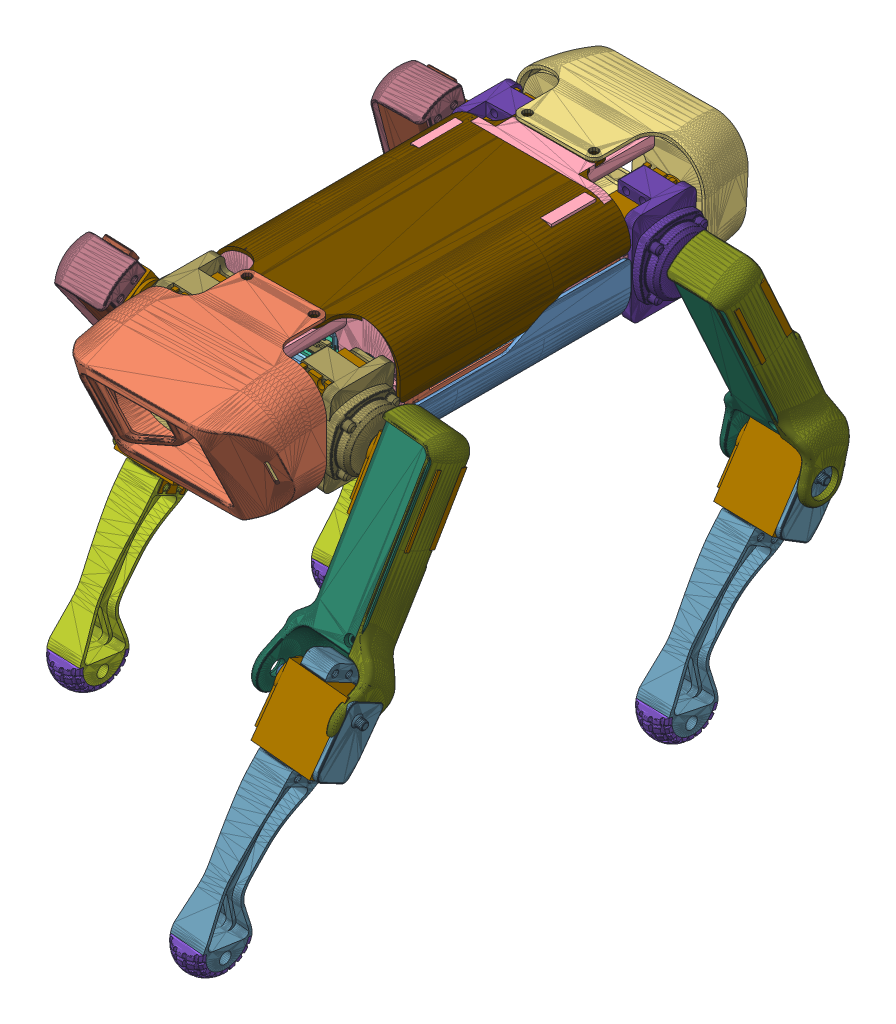
SolidWorks assembly robot_dog_jestson, configuration Default. Lengths in mm. (continued)
Components (placement in the parent): (continued)
- torsol_with_jestson-1: torsol_with_jestson [Default] at (84.8958 -47.9637 220.9974) size (110.41 70.14 242.41) (continued)
  - plate_with_jetson-1: plate_with_jetson [Default] at (-139.2728 38.0458 18.6623) x (-1 0 0) z (0 -1 0) size (107 130 44.9) (continued)
    - Jetson nano_fixed.step-1: Jetson nano_fixed.step [Default] at (-69.1681 -65.6237 -1.45) x (0 1 0) z (0 0 -1) size (100 81.03 30.51) (continued)
      - 142-13449-1000-A02_ASM.step-1: 142-13449-1000-A02_ASM.step [Default] at origin size (100 81.03 23.19) (continued)
        - 115-1821-000_1.step-2: 115-1821-000_1.step [Default] at (6.25 39.55 1.575) x (0 -1 0) z (0 0 1) size (2 2.88 1.1)
        - 115-0742-000_2.step-1: 115-0742-000_2.step [Default] at (3.05 46.85 1.575) size (2 2.88 1.1)
        - 115-0742-000_2.step-2: 115-0742-000_2.step [Default] at (3.05 51.65 1.575) x (-1 0 0) z (0 0 1) size (2 2.88 1.1)
        - 115-1821-000_1.step-3: 115-1821-000_1.step [Default] at (59.6 27.6 1.575) x (0 1 0) z (0 0 1) size (2 2.88 1.1)
        - 091-0022-000_1.step-1: 091-0022-000_1.step [Default] at (-0.95 5.7 1.575) size (2 2.51 1.1)
        - 091-0023-000_1.step-1: 091-0023-000_1.step [Default] at (15.25 29.9 1.575) x (0 -1 0) z (0 0 1) size (2 2.51 1.1)
        - 080-1368-000_1.step-1: 080-1368-000_1.step [Default] at (88 -14.3 1.575) size (10.99 7.28 4.95)
        - 080-1656-000_3.step-1: 080-1656-000_3.step [Default] at (44 16.6 1.575) x (-1 0 0) z (0 0 1) size (77.5 25.85 9.76)
        - 090-0243-000_1.step-1: 090-0243-000_1.step [Default] at (8.5 -4.1 1.575) x (-1 0 0) z (0 0 1) size (1.41 0.61 0.45)
        - 090-0243-000_1.step-2: 090-0243-000_1.step [Default] at (9.95 -3.7 1.575) x (0 1 0) z (0 0 1) size (1.41 0.61 0.45)
        - 090-0243-000_1.step-3: 090-0243-000_1.step [Default] at (9.5 -10.95 1.575) x (-1 0 0) z (0 0 1) size (1.41 0.61 0.45)
        - 090-0243-000_1.step-4: 090-0243-000_1.step [Default] at (9.8 -6.25 1.575) x (-1 0 0) z (0 0 1) size (1.41 0.61 0.45)
        - 090-0243-000_1.step-5: 090-0243-000_1.step [Default] at (9.5 -9.5 1.575) x (-1 0 0) z (0 0 1) size (1.41 0.61 0.45)
        - 090-0172-000_1.step-1: 090-0172-000_1.step [Default] at (90.6 -5 1.575) size (1.41 0.61 0.55)
        - 090-0172-000_1.step-2: 090-0172-000_1.step [Default] at (88.8 -5 1.575) x (-1 0 0) z (0 0 1) size (1.41 0.61 0.55)
        - 115-2177-000_2.step-1: 115-2177-000_2.step [Default] at (12.7 51.35 1.575) x (0 1 0) z (0 0 1) size (1.8 1.71 0.4)
        - 090-0233-000_1.step-1: 090-0233-000_1.step [Default] at (83.5 -6.6 1.575) size (3.3 1.3 0.74)
        - 064-0374-000_2.step-1: 064-0374-000_2.step [Default] at (19.75 -9.65 1.575) size (18.11 18.56 21.86)
        - 115-2628-000_3.step-1: 115-2628-000_3.step [Default] at (25.2 41.2 1.575) size (9.5 9.5 0.9)
        - 092-0073-000_1.step-1: 092-0073-000_1.step [Default] at (93.35 -4.75 1.575) x (-1 0 0) z (0 0 1) size (2.46 0.81 0.9)
        - IND_SMD_0402_H060.step-1: IND_SMD_0402_H060.step [Default] at (12.85 29.9 1.575) x (-1 0 0) z (0 0 1) size (1 0.5 0.6)
        - 1206_H190.step-1: 1206_H190.step [Default] at (82 18.8 1.575) x (0 1 0) z (0 0 1) size (3.2 1.6 1.9)
        - 1206_H190.step-2: 1206_H190.step [Default] at (81.95 13.5 1.575) x (0 -1 0) z (0 0 1) size (3.2 1.6 1.9)
        - 300-0868-000_3.step-1: 300-0868-000_3.step [Default] at (69.6 4 1.575) x (-1 0 0) z (0 0 1) size (1 0.6 0.4)
        - 300-0868-000_3.step-2: 300-0868-000_3.step [Default] at (9.55 0.95 1.575) size (1 0.6 0.4)
        - 300-0868-000_3.step-3: 300-0868-000_3.step [Default] at (19.6 31.45 1.575) x (0 -1 0) z (0 0 1) size (1 0.6 0.4)
        - 300-0868-000_3.step-4: 300-0868-000_3.step [Default] at (91.45 -2.45 1.575) x (-1 0 0) z (0 0 1) size (1 0.6 0.4)
        - 300-0868-000_3.step-5: 300-0868-000_3.step [Default] at (84.6 -5.1 1.575) size (1 0.6 0.4)
        - 300-0868-000_3.step-6: 300-0868-000_3.step [Default] at (66.725 5.875 1.575) x (0 -1 0) z (0 0 1) size (1 0.6 0.4)
        - 300-0868-000_3.step-7: 300-0868-000_3.step [Default] at (20.8 31.45 1.575) x (0 -1 0) z (0 0 1) size (1 0.6 0.4)
        - 300-0868-000_3.step-8: 300-0868-000_3.step [Default] at (62.9 31.35 1.575) x (-1 0 0) z (0 0 1) size (1 0.6 0.4)
        - 300-0868-000_3.step-9: 300-0868-000_3.step [Default] at (65.475 4.8 1.575) x (-1 0 0) z (0 0 1) size (1 0.6 0.4)
        - 300-0868-000_3.step-10: 300-0868-000_3.step [Default] at (63.9 33.85 1.575) x (-1 0 0) z (0 0 1) size (1 0.6 0.4)
        - 300-0868-000_3.step-11: 300-0868-000_3.step [Default] at (15.65 27.9 1.575) size (1 0.6 0.4)
        - 300-0868-000_3.step-12: 300-0868-000_3.step [Default] at (11.8 6.1 1.575) x (0 1 0) z (0 0 1) size (1 0.6 0.4)
        - 300-0868-000_3.step-13: 300-0868-000_3.step [Default] at (22.1 6.25 1.575) x (0 1 0) z (0 0 1) size (1 0.6 0.4)
        - 300-0869-000_3.step-1: 300-0869-000_3.step [Default] at (9.65 8.1 1.575) x (0 -1 0) z (0 0 1) size (1 0.6 0.53)
        - 300-0402-000_1.step-1: 300-0402-000_1.step [Default] at (20.8 26.45 1.575) x (0 -1 0) z (0 0 1) size (2 2.69 1.1)
        - 300-0560-000_1.step-1: 300-0560-000_1.step [Default] at (6.8 43.65 1.575) x (-1 0 0) z (0 0 1) size (2 2.69 1.1)
        - 174-0159-000_2.step-1: 174-0159-000_2.step [Default] at (61.49 57.15 1.575) x (-1 0 0) z (0 0 1) size (2 3.52 0.6)
        - 064-0373-000_2.step-1: 064-0373-000_2.step [Default] at (72.95 -7.825 1.575) size (17.8 21.61 17.46)
        - 064-0375-000_2.step-1: 064-0375-000_2.step [Default] at (19.751 -12.275 1.575) size (16.2 5.58 0.01)
        - 074-0221-000_3.step-1: 074-0221-000_3.step [Default] at (86 29 1.575) x (0 1 0) z (0 0 1) size (50.8 5.08 11.6)
        - 2016MM_H100.step-1: 2016MM_H100.step [Default] at (24.5 49.25 1.575) x (0 1 0) z (0 0 1) size (2 1.6 1)
        - 065-0656-000_2.step-1: 065-0656-000_2.step [Default] at (55.6 -10.04 1.575) x (-1 0 0) z (0 0 1) size (16.19 17.45 19.62)
        - 065-0656-000_2.step-2: 065-0656-000_2.step [Default] at (38.6 -10.04 1.575) x (-1 0 0) z (0 0 1) size (16.19 17.45 19.62)
        - 115-1921-000_3.step-1: 115-1921-000_3.step [Default] at (80.45 50.52 1.575) x (0 -1 0) z (0 0 1) size (5 4 1)
        - 115-1921-000_3.step-2: 115-1921-000_3.step [Default] at (80.4 34.5 1.575) x (0 -1 0) z (0 0 1) size (5 4 1)
        - 115-1921-000_3.step-3: 115-1921-000_3.step [Default] at (77.2 25.9 1.575) x (0 -1 0) z (0 0 1) size (5 4 1)
        - 085-0328-000_2.step-1: 085-0328-000_2.step [Default] at (16.28 36.32 1.575) x (0 -1 0) z (0 0 1) size (3.81 2.5 0.6)
        - 074-0216-000_2.step-1: 074-0216-000_2.step [Default] at (92.14 58 1.575) x (-1 0 0) z (0 0 1) size (4.83 5 11.5)
        - 060-0002-000_1.step-1: 060-0002-000_1.step [Default] at (41.2 57.9 1.575) x (0 -1 0) z (0 0 1) size (5.1 5.4 1.68)
        - 316-0697-000_1.step-1: 316-0697-000_1.step [Default] at (50.6 58.1 1.575) x (0 -1 0) z (0 0 1) size (3 3.72 0.8)
        - 032-0256-000_1.step-1: 032-0256-000_1.step [Default] at (5.925 9.425 1.575) size (4.22 2.82 2)
        - 041-0092-000_1.step-1: 041-0092-000_1.step [Default] at (46.9 54.9 1.575) x (0 -1 0) z (0 0 1) size (4.22 2.82 1.2)
        - 080-1243-000_3.step-1: 080-1243-000_3.step [Default] at (69.9 40.3 1.575) x (0 -1 0) z (0 0 1) size (21.9 9.1 4.8)
        - 102-0066-000_2.step-1: 102-0066-000_2.step [Default] at (18 4.2 1.575) size (1 1.86 0.61)
        - 102-0066-000_2.step-2: 102-0066-000_2.step [Default] at (13.55 4.2 1.575) size (1 1.86 0.61)
        - 102-0066-000_2.step-3: 102-0066-000_2.step [Default] at (32.45 5.81 1.575) size (1 1.86 0.61)
        - 102-0066-000_2.step-4: 102-0066-000_2.step [Default] at (27.65 5.81 1.575) size (1 1.86 0.61)
        - 102-0066-000_2.step-5: 102-0066-000_2.step [Default] at (20.15 4.2 1.575) size (1 1.86 0.61)
        - 102-0066-000_2.step-6: 102-0066-000_2.step [Default] at (15.75 4.2 1.575) size (1 1.86 0.61)
        - 102-0066-000_2.step-7: 102-0066-000_2.step [Default] at (29.25 5.81 1.575) size (1 1.86 0.61)
        - 102-0066-000_2.step-8: 102-0066-000_2.step [Default] at (30.85 5.81 1.575) size (1 1.86 0.61)
        - 102-0037-000_1.step-1: 102-0037-000_1.step [Default] at (55.2 2.95 1.575) x (-1 0 0) z (0 0 1) size (1 1.86 0.91)
        - 102-0037-000_1.step-2: 102-0037-000_1.step [Default] at (39.99 2.87 1.575) x (-1 0 0) z (0 0 1) size (1 1.86 0.91)
        - 102-0037-000_1.step-3: 102-0037-000_1.step [Default] at (60.55 2.95 1.575) x (-1 0 0) z (0 0 1) size (1 1.86 0.91)
        - 102-0037-000_1.step-4: 102-0037-000_1.step [Default] at (38.22 2.87 1.575) x (-1 0 0) z (0 0 1) size (1 1.86 0.91)
        - 0805_H140.step-1: 0805_H140.step [Default] at (8.1 -2.1 1.575) size (2.01 1.25 1.4)
        - 0805_H150.step-1: 0805_H150.step [Default] at (82.9 -8.4 1.575) x (-1 0 0) z (0 0 1) size (2.01 1.25 1.5)
        - 0603_H100.step-1: 0603_H100.step [Default] at (6.1 41.525 1.575) x (-1 0 0) z (0 0 1) size (1.6 0.81 1)
        - 0603_H060.step-1: 0603_H060.step [Default] at (63.25 -12 1.575) x (0 1 0) z (0 0 1) size (1.6 0.81 0.6)
        - 0603_H060.step-2: 0603_H060.step [Default] at (63.8 -0.7 1.575) x (0 -1 0) z (0 0 1) size (1.6 0.81 0.6)
        - 0603_H060.step-3: 0603_H060.step [Default] at (82.4 -10 1.575) x (-1 0 0) z (0 0 1) size (1.6 0.81 0.6)
        - 0603_H100.step-2: 0603_H100.step [Default] at (9.486 -7.5 1.575) x (-1 0 0) z (0 0 1) size (1.6 0.81 1)
        - 0603_H100.step-3: 0603_H100.step [Default] at (17.4 57.4 1.575) x (0 -1 0) z (0 0 1) size (1.6 0.81 1)
        - 0603_H100.step-4: 0603_H100.step [Default] at (30.35 25.9 1.575) x (0 -1 0) z (0 0 1) size (1.6 0.81 1)
        - 0603_H100.step-5: 0603_H100.step [Default] at (11.4 45.7 1.575) size (1.6 0.81 1)
        - 0603_H100.step-6: 0603_H100.step [Default] at (3.2 43 1.575) size (1.6 0.81 1)
        - 0603_H100.step-7: 0603_H100.step [Default] at (74.7 53.4 1.575) x (0 -1 0) z (0 0 1) size (1.6 0.81 1)
        - 0603_H100.step-8: 0603_H100.step [Default] at (69.5 53.9 1.575) x (0 -1 0) z (0 0 1) size (1.6 0.81 1)
        - 0603_H100.step-9: 0603_H100.step [Default] at (52.5 52.9 1.575) x (-1 0 0) z (0 0 1) size (1.6 0.81 1)
        - 0603_H100.step-10: 0603_H100.step [Default] at (52.5 54.2 1.575) x (-1 0 0) z (0 0 1) size (1.6 0.81 1)
        - 0603_H100.step-11: 0603_H100.step [Default] at (27.3 51.35 1.575) size (1.6 0.81 1)
        - 0603_H100.step-12: 0603_H100.step [Default] at (22.7 49.1 1.575) x (0 1 0) z (0 0 1) size (1.6 0.81 1)
        - 0603_H100.step-13: 0603_H100.step [Default] at (26.2 48.8 1.575) x (0 1 0) z (0 0 1) size (1.6 0.81 1)
        - 0603_H100.step-14: 0603_H100.step [Default] at (20.9 49.1 1.575) x (0 1 0) z (0 0 1) size (1.6 0.81 1)
        - 0603_H100.step-15: 0603_H100.step [Default] at (65.5 27.4 1.575) x (0 -1 0) z (0 0 1) size (1.6 0.81 1)
        - 0603_H100.step-16: 0603_H100.step [Default] at (63.8 52.2 1.575) x (-1 0 0) z (0 0 1) size (1.6 0.81 1)
        - 0603_H100.step-17: 0603_H100.step [Default] at (52.5 55.4 1.575) x (-1 0 0) z (0 0 1) size (1.6 0.81 1)
        - 080-1669-000_2.step-1: 080-1669-000_2.step [Default] at (0.2 29 1.575) x (0 -1 0) z (0 0 1) size (22.4 5.4 7.7)
      - 244-63448-0000-000_ASM.step-1: 244-63448-0000-000_ASM.step [Default] at (11.2 22.5 8.2712) size (69.6 45 21.37)
        - 142-13448-1000-A02_ASM.step-1: 142-13448-1000-A02_ASM.step [Default] at origin size (23 37.01 4.01)
          - 080-0051-000_3.step-1: 080-0051-000_3.step [Default] at (28.331 29.139 0) x (-1 0 0) z (0 0 -1) size (13.4 17 1.28)
          - TM670M-A2_1.step-1: TM670M-A2_1.step [Default] at (23.7 13.45 1.2) size (23 23 1.29)
        - 142-13448-1000-A02-SKU0000_ASM.step-1: 142-13448-1000-A02-SKU0000_ASM.step [Default] at origin size (23 23 1.29)
          - TM670M-A2_1.step-1: TM670M-A2_1.step [Default] at (23.7 13.45 1.2) size (23 23 1.29)
        - PORG_HSK_ASSY_ASM.step-1: PORG_HSK_ASSY_ASM.step [Default] at (0 0 4.01) size (58.7 39.4 17.3)
          - PORG_HEAT_SINK.step-1: PORG_HEAT_SINK.step [Default] at origin size (58.7 39.4 17.3)
        - 142-63448-1GEN_A00.step-1: 142-63448-1GEN_A00.step [Default] at origin size (69.6 45 1.2)
        - PORG_LEAF_SPRING_DRAWN.step-1: PORG_LEAF_SPRING_DRAWN.step [Default] at (0 0 -0.4) x (1 0.000001 0) z (0 0 1) size (39.83 21.3 1.2)
        - PORG_LEAF_SPRING_SCREW.step-1: PORG_LEAF_SPRING_SCREW.step [Default] at (6.9871 5.9982 5.21) x (0 0 -1) z (0 1 0) size (6.41 4.7 4.7)
        - PORG_LEAF_SPRING_SCREW.step-2: PORG_LEAF_SPRING_SCREW.step [Default] at (6.9871 20.9018 5.21) x (0 0 -1) z (0 1 0) size (6.41 4.7 4.7)
        - PORG_LEAF_SPRING_SCREW.step-3: PORG_LEAF_SPRING_SCREW.step [Default] at (40.4129 20.9018 5.21) x (0 0 -1) z (0 1 0) size (6.41 4.7 4.7)
        - PORG_LEAF_SPRING_SCREW.step-4: PORG_LEAF_SPRING_SCREW.step [Default] at (40.4129 5.9982 5.21) x (0 0 -1) z (0 1 0) size (6.41 4.7 4.7)
      - PORG_HEX_STANDOFF.step-1: PORG_HEX_STANDOFF.step [Default] at (75.8 58.5 8.17) x (-1 0 0) z (0 0 -1) size (5.14 4.45 6.57)
      - PORG_HEX_STANDOFF.step-2: PORG_HEX_STANDOFF.step [Default] at (12.2 58.5 8.17) x (-1 0 0) z (0 0 -1) size (5.14 4.45 6.57)
      - PORG_SYSTEM_SCREW.step-1: PORG_SYSTEM_SCREW.step [Default] at (12.2 58.5 3.73) size (4.55 4.55 4.53)
      - PORG_SYSTEM_SCREW.step-2: PORG_SYSTEM_SCREW.step [Default] at (75.8 58.5 3.73) size (4.55 4.55 4.53)
      - PORG_SYSTEM_SCREW.step-3: PORG_SYSTEM_SCREW.step [Default] at (75.8 58.5 5.67) x (-1 0 0) z (0 0 -1) size (4.55 4.55 4.53)
      - PORG_SYSTEM_SCREW.step-4: PORG_SYSTEM_SCREW.step [Default] at (12.2 58.5 5.67) x (-1 0 0) z (0 0 -1) size (4.55 4.55 4.53)
      - 155-0576-000.step-1: 155-0576-000.step [Default] at (40.276 40.3 5.01) size (5 5 4)
    - battery_4000mah_2s-1: battery_4000mah_2s [Default] at (-88.6681 58.3763 -1.45) x (1 0 0) z (0 -1 0) size (85 42 27)
  - copper_cylinder_jetson-1: copper_cylinder_jetson [Default] at (-70.1047 41.0708 -1.714) x (-0.061328 0 0.998118) z (0 1 0) size (3 3 30)
  - copper_cylinder_jetson-5: copper_cylinder_jetson [Default] at (-128.1047 71.0708 -1.714) x (0.951181 0 0.308634) z (0 -1 0) size (3 3 30)
  - copper_cylinder_jetson-6: copper_cylinder_jetson [Default] at (-128.1047 71.0708 84.286) x (0.479614 0 0.877479) z (0 -1 0) size (3 3 30)
  - copper_cylinder_jetson-7: copper_cylinder_jetson [Default] at (-70.1047 71.0708 84.286) x (-0.839782 0 0.542924) z (0 -1 0) size (3 3 30)
  - plate_top_jetson-1: plate_top_jetson [Default] at (-99.1047 74.0708 42.5512) x (-1 0 0) z (0 -1 0) size (66 94 3)
- right_foot_front-1: right_foot_front [Default] at (-126.7235 -93.0726 453.4039) x (-0.034309 -0.880659 0.472507) z (-0.018394 -0.472149 -0.881327) size (236.52 96.4 141.61) (flexible)
  - R_wrist_mg-1: R_wrist_mg [Default] at (-88.5645 -25.7472 139.9903) size (149.99 36.9 30)
  - foot-1: foot [Default] at (37.4355 -5.9472 149.9903) x (0.342021 0 -0.939692) z (-0.939692 0 -0.342021) size (38.32 20 19.41)
  - MG996R-1: MG996R [Default] at (-68.3145 3.2528 149.9903) x (1 0 0) z (0 0 -1) size (54.5 43 20)
    - servo-1: servo [Default] at origin size (54.5 39 20)
    - shaft-1: shaft [Default] at (-10.1089 43 0) x (-0.837169 0 -0.546944) z (-0.546944 0 0.837169) size (5.9 19.57 5.9)
  - R_arm_mg-1: R_arm_mg [Default] at (-134.0023 -85.7472 46.9151) x (-0.895965 0 0.444124) z (0.444124 0 0.895965) size (38.24 39.8 137.4)
  - MG996R-2: MG996R [Default] at (-133.9685 -3.7472 69.4996) x (0.444124 0 0.895965) z (0.895965 0 -0.444124) size (54.5 43 20)
    - servo-1: servo [Default] at origin size (54.5 39 20)
    - shaft-1: shaft [Default] at (-10.1089 43 0) x (-0.837169 0 -0.546944) z (-0.546944 0 0.837169) size (5.9 19.57 5.9)
  - R_arm_joint_mg-1: R_arm_joint_mg [Default] at (-161.1481 -115.2472 59.9077) x (0 -1 0) z (0.881327 0 0.472507) size (37.5 46 56.5)
  - R_arm_cover-1: R_arm_cover [Default] at (-129.9927 -48.0472 37.1147) x (-0.895965 0 0.444124) z (0.444124 0 0.895965) size (41.16 45 143.55)
  - MG996R-3: MG996R [Default] at (-146.1363 -75.2472 74.7639) x (0.881327 0 0.472507) z (0 1 0) size (54.5 43 20)
    - servo-1: servo [Default] at origin size (54.5 39 20)
    - shaft-1: shaft [Default] at (-10.1089 43 0) x (-0.837169 0 -0.546944) z (-0.546944 0 0.837169) size (5.9 19.57 5.9)
- left_foot_back-1: left_foot_back [Default] at (93.3781 -108.8977 296.0109) x (-0.021318 -0.848929 0.528077) z (-0.013257 -0.527911 -0.849196) size (284.28 93.4 85.82) (flexible)
  - L_wrist_mg-1: L_wrist_mg [Default] at (-104.9134 49.2874 139.9903) size (149.99 36.9 30)
  - foot-1: foot [Default] at (21.0866 19.2874 149.9903) x (0.342019 0 -0.939693) z (-0.939693 0 -0.342019) size (38.32 20 19.41)
  - MG996R-1: MG996R [Default] at (-84.6634 -9.7126 149.9903) size (54.5 43 20)
    - servo-1: servo [Default] at origin size (54.5 39 20)
    - shaft-1: shaft [Default] at (-10.1089 43 0) x (-0.837169 0 -0.546944) z (-0.546944 0 0.837169) size (5.9 19.57 5.9)
  - L_arm_mg-1: L_arm_mg [Default] at (-161.6203 26.2874 53.9721) x (-0.838875 0 0.544324) z (0.544324 0 0.838875) size (38.24 39.8 137.4)
  - MG996R-2: MG996R [Default] at (-158.9865 -5.7126 76.4026) x (0.544324 0 0.838875) z (-0.838875 0 0.544324) size (54.5 43 20)
    - servo-1: servo [Default] at origin size (54.5 39 20)
    - shaft-1: shaft [Default] at (-10.1089 43 0) x (-0.837169 0 -0.546944) z (-0.546944 0 0.837169) size (5.9 19.57 5.9)
  - L_arm_cover-1: L_arm_cover [Default] at (-160.8168 28.5874 45.1062) x (-0.838875 0 0.544324) z (0.544324 0 0.838875) size (41.16 45 143.55)
  - L_arm_joint_mg-1: L_arm_joint_mg [Default] at (-141.9481 74.7874 69.9359) x (0 -1 0) z (-0.849196 0 -0.528077) size (37.5 46 56.5)
  - MG996R-3: MG996R [Default] at (-156.825 65.7874 53.6191) x (0.849196 0 0.528077) z (0 -1 0) size (54.5 43 20)
    - servo-1: servo [Default] at origin size (54.5 39 20)
    - shaft-1: shaft [Default] at (-10.1089 43 0) x (-0.837169 0 -0.546944) z (-0.546944 0 0.837169) size (5.9 19.57 5.9)
- left_foot_front-1: left_foot_front [Default] at (86.019 -111.7023 568.2939) x (-0.086144 -0.870613 0.484368) z (-0.047693 -0.482014 -0.874864) size (271.86 94.6 110.14) (flexible)
  - L_wrist_mg-1: L_wrist_mg [Default] at (-104.9134 49.2874 139.9903) size (149.99 36.9 30)
  - foot-1: foot [Default] at (21.0866 19.2874 149.9903) x (0.342019 0 -0.939693) z (-0.939693 0 -0.342019) size (38.32 20 19.41)
  - MG996R-1: MG996R [Default] at (-84.6634 -9.7126 149.9903) size (54.5 43 20)
    - servo-1: servo [Default] at origin size (54.5 39 20)
    - shaft-1: shaft [Default] at (-10.1089 43 0) x (-0.837169 0 -0.546944) z (-0.546944 0 0.837169) size (5.9 19.57 5.9)
  - L_arm_mg-1: L_arm_mg [Default] at (-211.4877 30.2874 141.8872) x (-0.101729 0 0.994812) z (0.994812 0 0.101729) size (38.24 39.8 137.4)
  - MG996R-2: MG996R [Default] at (-192.3601 -1.7126 153.8953) x (0.994812 0 0.101729) z (-0.101729 0 0.994812) size (54.5 43 20)
    - servo-1: servo [Default] at origin size (54.5 39 20)
    - shaft-1: shaft [Default] at (-10.1089 43 0) x (-0.837169 0 -0.546944) z (-0.546944 0 0.837169) size (5.9 19.57 5.9)
  - L_arm_cover-1: L_arm_cover [Default] at (-217.8919 32.5874 135.7036) x (-0.101729 0 0.994812) z (0.994812 0 0.101729) size (41.16 45 143.55)
  - MG996R-3: MG996R [Default] at (-210.2875 66.9874 167.0835) x (0.874864 0 0.484368) z (0 1 0) size (54.5 43 20)
    - servo-1: servo [Default] at origin size (54.5 39 20)
    - shaft-1: shaft [Default] at (-10.1089 43 0) x (-0.837169 0 -0.546944) z (-0.546944 0 0.837169) size (5.9 19.57 5.9)
  - R_arm_joint_mg-1: R_arm_joint_mg [Default] at (-189.6653 106.9874 171.6427) x (0 1 0) z (-0.874864 0 -0.484368) size (37.5 46 56.5)
- right_foot_back-1: right_foot_back [Default] at (-115.1028 -105.3329 309.254) x (0.02206 -0.868899 0.494498) z (0.012551 -0.494339 -0.869179) size (200.98 91.6 160.78) (flexible)
  - R_wrist_mg-1: R_wrist_mg [Default] at (-88.5645 -25.7472 139.9903) size (149.99 36.9 30)
  - foot-1: foot [Default] at (37.4355 -5.9472 149.9903) x (0.342021 0 -0.939692) z (-0.939692 0 -0.342021) size (38.32 20 19.41)
  - MG996R-1: MG996R [Default] at (-68.3145 3.2528 149.9903) x (1 0 0) z (0 0 -1) size (54.5 43 20)
    - servo-1: servo [Default] at origin size (54.5 39 20)
    - shaft-1: shaft [Default] at (-10.1089 43 0) x (-0.837169 0 -0.546944) z (-0.546944 0 0.837169) size (5.9 19.57 5.9)
  - R_arm_mg-1: R_arm_mg [Default] at (-166.5461 -85.7472 72.8675) x (-0.684015 0 0.729468) z (0.729468 0 0.684015) size (38.24 39.8 137.4)
  - MG996R-2: MG996R [Default] at (-158.6145 -3.7472 94.0135) x (0.729468 0 0.684015) z (0.684015 0 -0.729468) size (54.5 43 20)
    - servo-1: servo [Default] at origin size (54.5 39 20)
    - shaft-1: shaft [Default] at (-10.1089 43 0) x (-0.837169 0 -0.546944) z (-0.546944 0 0.837169) size (5.9 19.57 5.9)
  - R_arm_cover-1: R_arm_cover [Default] at (-166.2178 -48.0472 62.2838) x (-0.684015 0 0.729468) z (0.729468 0 0.684015) size (41.16 45 143.55)
  - MG996R-3: MG996R [Default] at (-157.9418 -70.4472 73.046) x (0.869179 0 0.494498) z (0 -1 0) size (54.5 43 20)
    - servo-1: servo [Default] at origin size (54.5 39 20)
    - shaft-1: shaft [Default] at (-10.1089 43 0) x (-0.837169 0 -0.546944) z (-0.546944 0 0.837169) size (5.9 19.57 5.9)
  - L_arm_joint_mg-1: L_arm_joint_mg [Default] at (-178.5097 -80.4472 68.2475) x (0 1 0) z (0.869179 0 0.494498) size (37.5 46 56.5)
- non-mega_T_cover_mg-1: non-mega_T_cover_mg [Default] at (-65.4072 -90.53 364.1871) x (-0.004263 0.000801 -0.999991) z (0.999991 0 -0.004263) size (180 34.5 114)
- non-mega_B_cover_mg-1: non-mega_B_cover_mg [Default] at (-65.8721 -36.5293 363.9553) x (0 0.000778 -1) z (1 0 0) size (180 42.5 114)
- F_cover-1: F_cover [Default] at (48.4963 35.3945 333.4551) x (0.008769 -0.000778 0.999961) z (0 -1 -0.000778) size (92.81 114 70)
- R_cover-1: R_cover [Default] at (-66.43 33.5613 124.2887) x (-0.000003 -1 -0.000778) z (0.004263 -0.000778 0.999991) size (70 114 69.85)
Mates (geometry in assembly coordinates):
- Parallel2: parallel aligned: plane of torsol-1/O_shoulder-2 through (-63.7089 33.4959 362.262) normal (0 0 1); plane of right_foot_front-1/MG996R-3/shaft-1 through (-47.5013 7.4959 361.462) normal (0 0 1)
- Coincident9: coincident anti-aligned: line of torsol-1/O_shoulder-2 through (-47.5013 7.4959 362.262) axis (0 0 1); line of right_foot_front-1/MG996R-3/shaft-1 through (-47.5013 7.4959 361.462) axis (0 0 -1)
- Coincident10: coincident anti-aligned: plane of torsol-1/I_shoulder_mg-2 through (-63.7089 33.4959 313.962) normal (0 0 1); plane of right_foot_front-1/R_arm_joint_mg-1 through (-7.1368 16.0722 313.962) normal (0 0 -1)
- Coincident12: coincident anti-aligned: line of torsol-1/O_shoulder-1 through (30.4976 7.6867 125.662) axis (0 0 -1); line of left_foot_back-1/MG996R-3/shaft-1 through (30.4976 7.6867 124.662) axis (0 0 1)
- Distance3: distance = 1 mm aligned: plane of left_foot-1/MG996R-3/shaft-1 through (30.4976 7.6867 124.662) normal (0 0 -1); plane of torsol-1/O_shoulder-1 through (46.7052 33.6867 125.662) normal (0 0 -1)
- Coincident13: coincident anti-aligned: line of torsol-1/O_shoulder-2 through (30.4987 7.4959 362.262) axis (0 0 1); line of left_foot_front-1/MG996R-3/shaft-1 through (30.4987 7.4959 363.262) axis (0 0 -1)
- Distance4: distance = 1 mm aligned: plane of left_foot_front-1/MG996R-3/shaft-1 through (30.4987 7.4959 363.262) normal (0 0 1); plane of torsol-1/O_shoulder-2 through (-63.7089 33.4959 362.262) normal (0 0 1)
- Coincident15: coincident anti-aligned: line of torsol-1/O_shoulder-1 through (-47.5024 7.6867 125.662) axis (0 0 -1); line of right_foot_back-1/MG996R-3/shaft-1 through (-47.5024 7.6867 124.662) axis (0 0 1)
- Distance5: distance = 1 mm aligned: plane of right_foot_back-1/MG996R-3/shaft-1 through (-47.5024 7.6867 124.662) normal (0 0 -1); plane of torsol-1/O_shoulder-1 through (46.7052 33.6867 125.662) normal (0 0 -1)
- Coincident19: coincident: point of torsol-1/I_shoulder_mg-2; point of non-mega_T_cover_mg-1
- Coincident20: coincident: line of torsol-1/I_shoulder_mg-2 through (-29.1961 31.4959 331.516) axis (-0.951057 0 -0.309017); point of non-mega_T_cover_mg-1
- Coincident22: coincident: plane of torsol-1/I_shoulder_mg-1 through (46.2911 31.6321 178.962) normal (0 1 0); point of non-mega_T_cover_mg-1
- Coincident23: coincident: point of torsol-1/I_shoulder_mg-2; point of non-mega_B_cover_mg-1
- Coincident24: coincident: line of torsol-1/I_shoulder_mg-2 through (-3.2217 -34.5041 331.516) axis (-0.998027 0 0.06279); point of non-mega_B_cover_mg-1
- Coincident25: coincident: plane of torsol-1/I_shoulder_mg-1 through (46.2911 -34.3679 178.962) normal (0 -1 0); point of non-mega_B_cover_mg-1
- Coincident26: coincident: point of non-mega_T_cover_mg-1; point of F_cover-1
- Coincident27: coincident: line of non-mega_T_cover_mg-1 through (12.1055 33.5 326.4443) axis (-0.991992 0.000105 -0.126301); point of F_cover-1
- Parallel5: parallel anti-aligned: plane of non-mega_B_cover_mg-1 through (-65.8721 -36.5293 363.9553) normal (0 -1 -0.000778); plane of F_cover-1 through (48.4963 -32.7055 333.4021) normal (0 1 0.000778)
- Coincident31: coincident: point of non-mega_T_cover_mg-1; point of R_cover-1
- Coincident32: coincident: line of non-mega_T_cover_mg-1 through (-29.9433 33.6321 161.6449) axis (0.991993 -0.000105 0.12629); point of R_cover-1
